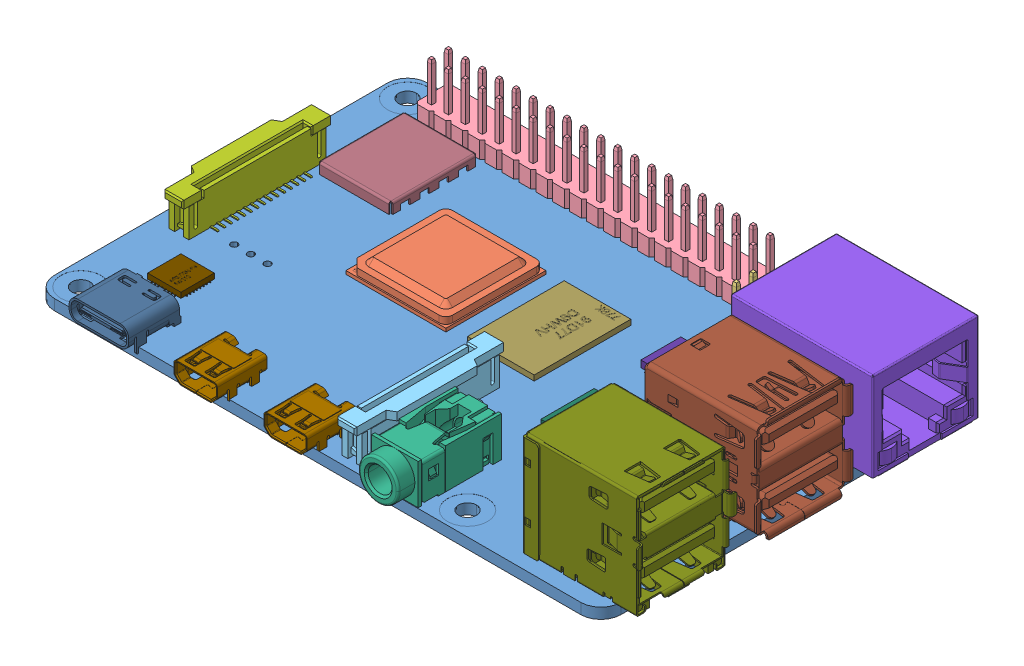
SolidWorks assembly Raspberry Pi 4 Model B, configuration Default. Lengths in mm.
Overall size (89 19.92 58.4).
20 component instances, 18 part files, 0 mates.
Components (placement in the parent):
- Raspberry Pi 4 Model B.STEP-1: Raspberry Pi 4 Model B.STEP [Default] at origin size (89 19.92 58.4)
  - PCB, RPi4ModelB.STEP-1: PCB, RPi4ModelB.STEP [Default] at origin size (85 1.6 56)
  - Broadcom BCM2711B0 CPU, RPi4ModelB.STEP-1: Broadcom BCM2711B0 CPU, RPi4ModelB.STEP [Default] at (-13.25 0.8 -4.5) size (15 2.3 15)
  - 2.54 mm DUPONT MALE PIN HEADER, POE, 2X2, RPi4ModelB.STEP-1: 2.54 mm DUPONT MALE PIN HEADER, POE, 2X2, RPi4ModelB.STEP [Default] at (19 0.8 -18.36) size (5.08 11.3 5.08)
  - 2.54 mm DUPONT MALE PIN HEADER, IO, 2X20, RPi4ModelB.STEP-1: 2.54 mm DUPONT MALE PIN HEADER, IO, 2X20, RPi4ModelB.STEP [Default] at (-10 0.8 -24.5) size (50.8 11.3 5.08)
  - Camera Connector, RPi4ModelB.STEP-1: Camera Connector, RPi4ModelB.STEP [Default] at (4 0.8 16.5) x (0 0 -1) z (1 0 0) size (22.4 5.68 5.07)
  - Microphone Plug, RPi4ModelB.STEP-1: Microphone Plug, RPi4ModelB.STEP [Default] at (11.5 0.8 21.65) size (7.23 7.55 15)
  - Display Connector, RPi4ModelB.STEP-1: Display Connector, RPi4ModelB.STEP [Default] at (-38.5 0.8 0) x (0 0 1) z (-1 0 0) size (22.4 5.68 5.07)
  - Gigabit Ethernet Port, RPi4ModelB.STEP-1: Gigabit Ethernet Port, RPi4ModelB.STEP [Default] at (45.5 7.55 -17.75) x (0 0 -1) z (1 0 0) size (16.33 17.24 21.6)
  - Female Micro HDMI Connector, RPi4ModelB.STEP-1: Female Micro HDMI Connector, RPi4ModelB.STEP [Default] at (-3 0.8 27.3875) size (6.5 3.51 7.5)
  - Female Micro HDMI Connector, RPi4ModelB.STEP-2: Female Micro HDMI Connector, RPi4ModelB.STEP [Default] at (-16.5 0.8 27.3875) size (6.5 3.51 7.5)
  - Female USB Type C Connector, RPi4ModelB.STEP-1: Female USB Type C Connector, RPi4ModelB.STEP [Default] at (-31.3 0.8 26.5419) size (8.94 3.96 7.9)
  - 2X USB3.0 PORTS, RPi4ModelB.STEP-1: 2X USB3.0 PORTS, RPi4ModelB.STEP [Default] at (37.07 0.8 1) size (17.48 19.42 15.69)
  - 91D77 D9WHV 778K, 4 GB LPDDR4 SDRAM, RPi4ModelB.STEP-1: 91D77 D9WHV 778K, 4 GB LPDDR4 SDRAM, RPi4ModelB.STEP [Default] at (2.25 0.8 -4.5) size (10 0.8 14.5)
  - Cypress CYW43455 Wireless Module Cover, RPi4ModelB.STEP-1: Cypress CYW43455 Wireless Module Cover, RPi4ModelB.STEP [Default] at (-30.5 0.8 -14.5) size (11 1.6 13)
  - SD Card Slot, RPi4ModelB.STEP-1: SD Card Slot, RPi4ModelB.STEP [Default] at (-35.3 -0.8 0) x (0 0 -1) z (-1 0 0) size (11.95 1.45 11.4)
  - VIA VL805 PCIe USB 3.0 controller, RPi4ModelB.STEP-1: VIA VL805 PCIe USB 3.0 controller, RPi4ModelB.STEP [Default] at (17.5 0.8 4) size (8.8 0.8 8.8)
  - 2X USB2.0 PORTS, RPi4ModelB.STEP-1: 2X USB2.0 PORTS, RPi4ModelB.STEP [Default] at (37.065 0.65 19) size (17.87 19.17 15.35)
  - Broadcom BCM54213PE Gigabit Ethernet Transceiver, RPi4ModelB.STEP-1: Broadcom BCM54213PE Gigabit Ethernet Transceiver, RPi4ModelB.STEP [Default] at (16.5 0.8 -10) size (6.8 1 6.8)
  - MxL7704 Universal PMIC, RPi4ModelB.STEP-1: MxL7704 Universal PMIC, RPi4ModelB.STEP [Default] at (-32.5 0.8 16) size (5.4 0.8 5.4)
